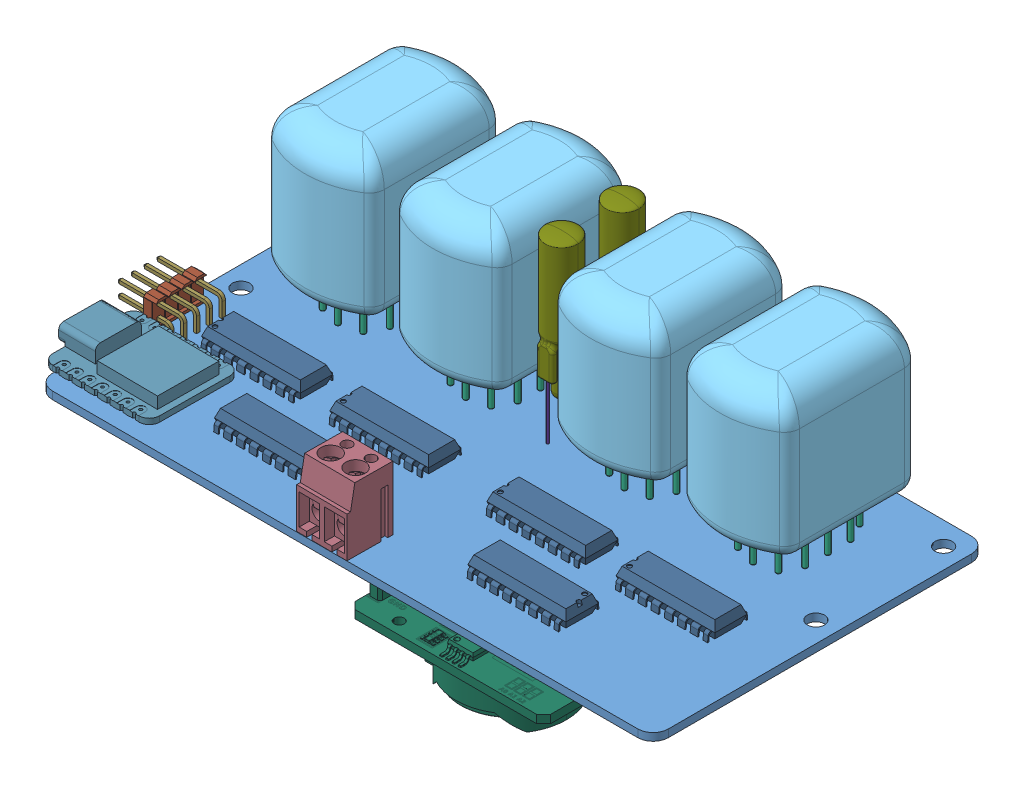
SolidWorks assembly board, configuration Défaut. Lengths in mm.
Overall size (127.16 50.53 67.27).
290 component instances, 53 part files, 23 mates.
Components (placement in the parent):
- pcb-1: pcb [Défaut] at origin size (121.6 1.5 65.9)
- IN-12A.stp-1: IN-12A.stp [Défaut] at (-40.9487 32.5 -15.5981) x (0 1 0) z (1 0 0) size (35 31 21)
  - 2.stp-1: 2.stp [Défaut] at origin size (2.7 24.17 15.83)
  - 3.stp-1: 3.stp [Défaut] at (-12.2 0 0) x (0 0 -1) z (-1 0 0) size (2 1.5 18.5)
  - 4.stp-1: 4.stp [Défaut] at (-12.2 0 0) x (0 0 1) z (-1 0 0) size (2 1.5 18.5)
  - 5.stp-1: 5.stp [Défaut] at (-12 0 0) x (0 0 -1) z (1 0 0) size (2.1 2.1 1)
  - 5.stp-2: 5.stp [Défaut] at (-10.8 0 0) x (0 0 -1) z (1 0 0) size (2.1 2.1 1)
  - 5.stp-3: 5.stp [Défaut] at (-9.6 0 0) x (0 0 -1) z (1 0 0) size (2.1 2.1 1)
  - 5.stp-4: 5.stp [Défaut] at (-8.4 0 0) x (0 0 -1) z (1 0 0) size (2.1 2.1 1)
  - 5.stp-5: 5.stp [Défaut] at (-7.2 0 0) x (0 0 -1) z (1 0 0) size (2.1 2.1 1)
  - 5.stp-6: 5.stp [Défaut] at (-6 0 0) x (0 0 -1) z (1 0 0) size (2.1 2.1 1)
  - 5.stp-7: 5.stp [Défaut] at (-4.8 0 0) x (0 0 -1) z (1 0 0) size (2.1 2.1 1)
  - 5.stp-8: 5.stp [Défaut] at (-3.6 0 0) x (0 0 -1) z (1 0 0) size (2.1 2.1 1)
  - 5.stp-9: 5.stp [Défaut] at (-2.4 0 0) x (0 0 -1) z (1 0 0) size (2.1 2.1 1)
  - 5.stp-10: 5.stp [Défaut] at (-1.2 0 0) x (0 0 -1) z (1 0 0) size (2.1 2.1 1)
  - 6.stp-1: 6.stp [Défaut] at (-11 16.1596 7.8778) x (0 -0.787778 0.61596) z (-1 0 0) size (2.1 2.1 1)
  - 7.stp-1: 7.stp [Défaut] at (-9.8 16.1596 7.8778) x (0 -0.787778 0.61596) z (-1 0 0) size (2.1 2.1 1)
  - 8.stp-1: 8.stp [Défaut] at (-8.6 16.1596 7.8778) x (0 -0.787778 0.61596) z (-1 0 0) size (2.1 2.1 1)
  - 9.stp-1: 9.stp [Défaut] at (-7.4 16.1596 7.8778) x (0 -0.787778 0.61596) z (-1 0 0) size (2.1 2.1 1)
  - 10.stp-1: 10.stp [Défaut] at (-6.2 16.1596 7.8778) x (0 -0.787778 0.61596) z (-1 0 0) size (2.1 2.1 1)
  - 11.stp-1: 11.stp [Défaut] at (-5 16.1596 7.8778) x (0 -0.787778 0.61596) z (-1 0 0) size (2.1 2.1 1)
  - 12.stp-1: 12.stp [Défaut] at (-3.8 16.1596 7.8778) x (0 -0.787778 0.61596) z (-1 0 0) size (2.1 2.1 1)
  - 13.stp-1: 13.stp [Défaut] at (-2.6 16.1596 7.8778) x (0 -0.787778 0.61596) z (-1 0 0) size (2.1 2.1 1)
  - 14.stp-1: 14.stp [Défaut] at (-1.4 16.1596 7.8778) x (0 -0.787778 0.61596) z (-1 0 0) size (2.1 2.1 1)
  - 15.stp-1: 15.stp [Défaut] at (-0.2 16.1596 7.8778) x (0 -0.787778 0.61596) z (-1 0 0) size (2.1 2.1 1)
  - 5.stp-11: 5.stp [Défaut] x (0 0 -1) z (1 0 0) size (2.1 2.1 1)
  - 5.stp-12: 5.stp [Défaut] at (-13.2 0 0) x (0 0 -1) z (1 0 0) size (2.1 2.1 1)
  - 16.stp-1: 16.stp [Défaut] at (1 16.1596 7.8778) x (0 -0.787778 0.61596) z (-1 0 0) size (2.1 2.1 1)
  - 17.stp-1: 17.stp [Défaut] at (-12.2 16.1596 7.8778) x (0 -0.787778 0.61596) z (-1 0 0) size (2.1 2.1 1)
  - 18.stp-1: 18.stp [Défaut] at (-13.2 0 0) x (0 0 -1) z (-1 0 0) size (15.83 24.17 12.28)
  - 19.stp-1: 19.stp [Défaut] x (1 0 0) z (0 1 0) size (1.51 1.46 20.68)
  - 20.stp-1: 20.stp [Défaut] at (1 0 0) size (4 22.27 2.42)
  - 21.stp-1: 21.stp [Défaut] at (-13.4 0 0) x (0 0 -1) z (-1 0 0) size (15.83 24.17 1)
  - 22.stp-1: 22.stp [Défaut] at (-14.4 0 0) x (0 0 -1) z (-1 0 0) size (15.83 27.29 2)
  - 23.stp-1: 23.stp [Défaut] x (0 0 -1) z (-1 0 0) size (21 31 33)
  - 24.stp-1: 24.stp [Défaut] x (0 0 -1) z (-1 0 0) size (1 1 15.5)
  - 24.stp-2: 24.stp [Défaut] at (0 -4.5 0) x (0 0 -1) z (-1 0 0) size (1 1 15.5)
  - 24.stp-3: 24.stp [Défaut] at (0 -8 -1.75) x (0 0 -1) z (-1 0 0) size (1 1 15.5)
  - 24.stp-4: 24.stp [Défaut] at (0 -9 -5.75) x (0 0 -1) z (-1 0 0) size (1 1 15.5)
  - 24.stp-5: 24.stp [Défaut] at (0 -8 -9.75) x (0 0 -1) z (-1 0 0) size (1 1 15.5)
  - 24.stp-6: 24.stp [Défaut] at (0 -4.5 -11.5) x (0 0 -1) z (-1 0 0) size (1 1 15.5)
  - 24.stp-7: 24.stp [Défaut] at (0 0 -11.5) x (0 0 -1) z (-1 0 0) size (1 1 15.5)
  - 24.stp-8: 24.stp [Défaut] at (0 4.5 -11.5) x (0 0 -1) z (-1 0 0) size (1 1 15.5)
  - 24.stp-9: 24.stp [Défaut] at (0 8 -9.75) x (0 0 -1) z (-1 0 0) size (1 1 15.5)
  - 24.stp-10: 24.stp [Défaut] at (0 9 -5.75) x (0 0 -1) z (-1 0 0) size (1 1 15.5)
  - 24.stp-11: 24.stp [Défaut] at (0 8 -1.75) x (0 0 -1) z (-1 0 0) size (1 1 15.5)
  - 24.stp-12: 24.stp [Défaut] at (0 4.5 0) x (0 0 -1) z (-1 0 0) size (1 1 15.5)
  - 25.stp-1: 25.stp [Défaut] at (-1.4 0 0) x (0 0 1) z (1 0 0) size (10.55 22 0.2)
  - 26.stp-1: 26.stp [Défaut] at (-2.6 0 0) x (0 0 1) z (1 0 0) size (11 22 0.2)
  - 27.stp-1: 27.stp [Défaut] at (-3.8 0 0) x (0 0 1) z (1 0 0) size (11 22 0.2)
  - 28.stp-1: 28.stp [Défaut] at (-5 0 0) x (0 0 1) z (1 0 0) size (10 22 0.2)
  - 29.stp-1: 29.stp [Défaut] at (-7.4 0 0) x (0 0 1) z (1 0 0) size (10 22 0.2)
  - 30.stp-1: 30.stp [Défaut] at (-9.6 0 0) x (0 0 -1) z (-1 0 0) size (10 22 0.2)
  - 31.stp-1: 31.stp [Défaut] at (-11 0 0) x (0 0 1) z (1 0 0) size (11 22 0.2)
  - 32.stp-1: 32.stp [Défaut] at (-12.2 0 0) x (0 0 1) z (1 0 0) size (2 22 0.2)
  - 33.stp-1: 33.stp [Défaut] at (-6 0 0) x (0 0 -1) z (-1 0 0) size (11 22 0.2)
  - 34.stp-1: 34.stp [Défaut] at (-8.6 0 0) x (0 0 1) z (1 0 0) size (10 22 0.2)
  - 1.stp-1: 1.stp [Défaut] at origin size (7.54 3.19 3.19)
  - 1-0.stp-1: 1-0.stp [Défaut] at origin size (11.99 9.11 6.32)
  - 1-1.stp-1: 1-1.stp [Défaut] at origin size (5.03 4.26 4.61)
  - 1-2.stp-1: 1-2.stp [Défaut] at origin size (8.17 8.42 6.65)
  - 1-3.stp-1: 1-3.stp [Défaut] at origin size (17.22 12.89 7.69)
  - 1-4.stp-1: 1-4.stp [Défaut] at origin size (13.11 12.81 7.39)
  - 1-5.stp-1: 1-5.stp [Défaut] at origin size (15.91 7.54 6.9)
  - 1-6.stp-1: 1-6.stp [Défaut] at origin size (10.39 4.47 4.23)
  - 1-7.stp-1: 1-7.stp [Défaut] at origin size (7.32 4.98 2.44)
  - 1-8.stp-1: 1-8.stp [Défaut] at origin size (10.29 4.36 5.63)
  - 1-9.stp-1: 1-9.stp [Défaut] at origin size (12.89 8.1 7.83)
- IN-12A.stp-2: IN-12A.stp [Défaut] at (15.5408 32.5 -15.6508) x (0 1 0) z (1 0 0) size (35 31 21)
  - 2.stp-1: 2.stp [Défaut] at origin size (2.7 24.17 15.83)
  - 3.stp-1: 3.stp [Défaut] at (-12.2 0 0) x (0 0 -1) z (-1 0 0) size (2 1.5 18.5)
  - 4.stp-1: 4.stp [Défaut] at (-12.2 0 0) x (0 0 1) z (-1 0 0) size (2 1.5 18.5)
  - 5.stp-1: 5.stp [Défaut] at (-12 0 0) x (0 0 -1) z (1 0 0) size (2.1 2.1 1)
  - 5.stp-2: 5.stp [Défaut] at (-10.8 0 0) x (0 0 -1) z (1 0 0) size (2.1 2.1 1)
  - 5.stp-3: 5.stp [Défaut] at (-9.6 0 0) x (0 0 -1) z (1 0 0) size (2.1 2.1 1)
  - 5.stp-4: 5.stp [Défaut] at (-8.4 0 0) x (0 0 -1) z (1 0 0) size (2.1 2.1 1)
  - 5.stp-5: 5.stp [Défaut] at (-7.2 0 0) x (0 0 -1) z (1 0 0) size (2.1 2.1 1)
  - 5.stp-6: 5.stp [Défaut] at (-6 0 0) x (0 0 -1) z (1 0 0) size (2.1 2.1 1)
  - 5.stp-7: 5.stp [Défaut] at (-4.8 0 0) x (0 0 -1) z (1 0 0) size (2.1 2.1 1)
  - 5.stp-8: 5.stp [Défaut] at (-3.6 0 0) x (0 0 -1) z (1 0 0) size (2.1 2.1 1)
  - 5.stp-9: 5.stp [Défaut] at (-2.4 0 0) x (0 0 -1) z (1 0 0) size (2.1 2.1 1)
  - 5.stp-10: 5.stp [Défaut] at (-1.2 0 0) x (0 0 -1) z (1 0 0) size (2.1 2.1 1)
  - 6.stp-1: 6.stp [Défaut] at (-11 16.1596 7.8778) x (0 -0.787778 0.61596) z (-1 0 0) size (2.1 2.1 1)
  - 7.stp-1: 7.stp [Défaut] at (-9.8 16.1596 7.8778) x (0 -0.787778 0.61596) z (-1 0 0) size (2.1 2.1 1)
  - 8.stp-1: 8.stp [Défaut] at (-8.6 16.1596 7.8778) x (0 -0.787778 0.61596) z (-1 0 0) size (2.1 2.1 1)
  - 9.stp-1: 9.stp [Défaut] at (-7.4 16.1596 7.8778) x (0 -0.787778 0.61596) z (-1 0 0) size (2.1 2.1 1)
  - 10.stp-1: 10.stp [Défaut] at (-6.2 16.1596 7.8778) x (0 -0.787778 0.61596) z (-1 0 0) size (2.1 2.1 1)
  - 11.stp-1: 11.stp [Défaut] at (-5 16.1596 7.8778) x (0 -0.787778 0.61596) z (-1 0 0) size (2.1 2.1 1)
  - 12.stp-1: 12.stp [Défaut] at (-3.8 16.1596 7.8778) x (0 -0.787778 0.61596) z (-1 0 0) size (2.1 2.1 1)
  - 13.stp-1: 13.stp [Défaut] at (-2.6 16.1596 7.8778) x (0 -0.787778 0.61596) z (-1 0 0) size (2.1 2.1 1)
  - 14.stp-1: 14.stp [Défaut] at (-1.4 16.1596 7.8778) x (0 -0.787778 0.61596) z (-1 0 0) size (2.1 2.1 1)
  - 15.stp-1: 15.stp [Défaut] at (-0.2 16.1596 7.8778) x (0 -0.787778 0.61596) z (-1 0 0) size (2.1 2.1 1)
  - 5.stp-11: 5.stp [Défaut] x (0 0 -1) z (1 0 0) size (2.1 2.1 1)
  - 5.stp-12: 5.stp [Défaut] at (-13.2 0 0) x (0 0 -1) z (1 0 0) size (2.1 2.1 1)
  - 16.stp-1: 16.stp [Défaut] at (1 16.1596 7.8778) x (0 -0.787778 0.61596) z (-1 0 0) size (2.1 2.1 1)
  - 17.stp-1: 17.stp [Défaut] at (-12.2 16.1596 7.8778) x (0 -0.787778 0.61596) z (-1 0 0) size (2.1 2.1 1)
  - 18.stp-1: 18.stp [Défaut] at (-13.2 0 0) x (0 0 -1) z (-1 0 0) size (15.83 24.17 12.28)
  - 19.stp-1: 19.stp [Défaut] x (1 0 0) z (0 1 0) size (1.51 1.46 20.68)
  - 20.stp-1: 20.stp [Défaut] at (1 0 0) size (4 22.27 2.42)
  - 21.stp-1: 21.stp [Défaut] at (-13.4 0 0) x (0 0 -1) z (-1 0 0) size (15.83 24.17 1)
  - 22.stp-1: 22.stp [Défaut] at (-14.4 0 0) x (0 0 -1) z (-1 0 0) size (15.83 27.29 2)
  - 23.stp-1: 23.stp [Défaut] x (0 0 -1) z (-1 0 0) size (21 31 33)
  - 24.stp-1: 24.stp [Défaut] x (0 0 -1) z (-1 0 0) size (1 1 15.5)
  - 24.stp-2: 24.stp [Défaut] at (0 -4.5 0) x (0 0 -1) z (-1 0 0) size (1 1 15.5)
  - 24.stp-3: 24.stp [Défaut] at (0 -8 -1.75) x (0 0 -1) z (-1 0 0) size (1 1 15.5)
  - 24.stp-4: 24.stp [Défaut] at (0 -9 -5.75) x (0 0 -1) z (-1 0 0) size (1 1 15.5)
  - 24.stp-5: 24.stp [Défaut] at (0 -8 -9.75) x (0 0 -1) z (-1 0 0) size (1 1 15.5)
  - 24.stp-6: 24.stp [Défaut] at (0 -4.5 -11.5) x (0 0 -1) z (-1 0 0) size (1 1 15.5)
  - 24.stp-7: 24.stp [Défaut] at (0 0 -11.5) x (0 0 -1) z (-1 0 0) size (1 1 15.5)
  - 24.stp-8: 24.stp [Défaut] at (0 4.5 -11.5) x (0 0 -1) z (-1 0 0) size (1 1 15.5)
  - 24.stp-9: 24.stp [Défaut] at (0 8 -9.75) x (0 0 -1) z (-1 0 0) size (1 1 15.5)
  - 24.stp-10: 24.stp [Défaut] at (0 9 -5.75) x (0 0 -1) z (-1 0 0) size (1 1 15.5)
  - 24.stp-11: 24.stp [Défaut] at (0 8 -1.75) x (0 0 -1) z (-1 0 0) size (1 1 15.5)
  - 24.stp-12: 24.stp [Défaut] at (0 4.5 0) x (0 0 -1) z (-1 0 0) size (1 1 15.5)
  - 25.stp-1: 25.stp [Défaut] at (-1.4 0 0) x (0 0 1) z (1 0 0) size (10.55 22 0.2)
  - 26.stp-1: 26.stp [Défaut] at (-2.6 0 0) x (0 0 1) z (1 0 0) size (11 22 0.2)
  - 27.stp-1: 27.stp [Défaut] at (-3.8 0 0) x (0 0 1) z (1 0 0) size (11 22 0.2)
  - 28.stp-1: 28.stp [Défaut] at (-5 0 0) x (0 0 1) z (1 0 0) size (10 22 0.2)
  - 29.stp-1: 29.stp [Défaut] at (-7.4 0 0) x (0 0 1) z (1 0 0) size (10 22 0.2)
  - 30.stp-1: 30.stp [Défaut] at (-9.6 0 0) x (0 0 -1) z (-1 0 0) size (10 22 0.2)
  - 31.stp-1: 31.stp [Défaut] at (-11 0 0) x (0 0 1) z (1 0 0) size (11 22 0.2)
  - 32.stp-1: 32.stp [Défaut] at (-12.2 0 0) x (0 0 1) z (1 0 0) size (2 22 0.2)
  - 33.stp-1: 33.stp [Défaut] at (-6 0 0) x (0 0 -1) z (-1 0 0) size (11 22 0.2)
  - 34.stp-1: 34.stp [Défaut] at (-8.6 0 0) x (0 0 1) z (1 0 0) size (10 22 0.2)
  - 1.stp-1: 1.stp [Défaut] at origin size (7.54 3.19 3.19)
  - 1-0.stp-1: 1-0.stp [Défaut] at origin size (11.99 9.11 6.32)
  - 1-1.stp-1: 1-1.stp [Défaut] at origin size (5.03 4.26 4.61)
  - 1-2.stp-1: 1-2.stp [Défaut] at origin size (8.17 8.42 6.65)
  - 1-3.stp-1: 1-3.stp [Défaut] at origin size (17.22 12.89 7.69)
  - 1-4.stp-1: 1-4.stp [Défaut] at origin size (13.11 12.81 7.39)
  - 1-5.stp-1: 1-5.stp [Défaut] at origin size (15.91 7.54 6.9)
  - 1-6.stp-1: 1-6.stp [Défaut] at origin size (10.39 4.47 4.23)
  - 1-7.stp-1: 1-7.stp [Défaut] at origin size (7.32 4.98 2.44)
  - 1-8.stp-1: 1-8.stp [Défaut] at origin size (10.29 4.36 5.63)
  - 1-9.stp-1: 1-9.stp [Défaut] at origin size (12.89 8.1 7.83)
- IN-12A.stp-3: IN-12A.stp [Défaut] at (-15.577 32.5 -15.4564) x (0 1 0) z (1 0 0) size (35 31 21)
  - 2.stp-1: 2.stp [Défaut] at origin size (2.7 24.17 15.83)
  - 3.stp-1: 3.stp [Défaut] at (-12.2 0 0) x (0 0 -1) z (-1 0 0) size (2 1.5 18.5)
  - 4.stp-1: 4.stp [Défaut] at (-12.2 0 0) x (0 0 1) z (-1 0 0) size (2 1.5 18.5)
  - 5.stp-1: 5.stp [Défaut] at (-12 0 0) x (0 0 -1) z (1 0 0) size (2.1 2.1 1)
  - 5.stp-2: 5.stp [Défaut] at (-10.8 0 0) x (0 0 -1) z (1 0 0) size (2.1 2.1 1)
  - 5.stp-3: 5.stp [Défaut] at (-9.6 0 0) x (0 0 -1) z (1 0 0) size (2.1 2.1 1)
  - 5.stp-4: 5.stp [Défaut] at (-8.4 0 0) x (0 0 -1) z (1 0 0) size (2.1 2.1 1)
  - 5.stp-5: 5.stp [Défaut] at (-7.2 0 0) x (0 0 -1) z (1 0 0) size (2.1 2.1 1)
  - 5.stp-6: 5.stp [Défaut] at (-6 0 0) x (0 0 -1) z (1 0 0) size (2.1 2.1 1)
  - 5.stp-7: 5.stp [Défaut] at (-4.8 0 0) x (0 0 -1) z (1 0 0) size (2.1 2.1 1)
  - 5.stp-8: 5.stp [Défaut] at (-3.6 0 0) x (0 0 -1) z (1 0 0) size (2.1 2.1 1)
  - 5.stp-9: 5.stp [Défaut] at (-2.4 0 0) x (0 0 -1) z (1 0 0) size (2.1 2.1 1)
  - 5.stp-10: 5.stp [Défaut] at (-1.2 0 0) x (0 0 -1) z (1 0 0) size (2.1 2.1 1)
  - 6.stp-1: 6.stp [Défaut] at (-11 16.1596 7.8778) x (0 -0.787778 0.61596) z (-1 0 0) size (2.1 2.1 1)
  - 7.stp-1: 7.stp [Défaut] at (-9.8 16.1596 7.8778) x (0 -0.787778 0.61596) z (-1 0 0) size (2.1 2.1 1)
  - 8.stp-1: 8.stp [Défaut] at (-8.6 16.1596 7.8778) x (0 -0.787778 0.61596) z (-1 0 0) size (2.1 2.1 1)
  - 9.stp-1: 9.stp [Défaut] at (-7.4 16.1596 7.8778) x (0 -0.787778 0.61596) z (-1 0 0) size (2.1 2.1 1)
  - 10.stp-1: 10.stp [Défaut] at (-6.2 16.1596 7.8778) x (0 -0.787778 0.61596) z (-1 0 0) size (2.1 2.1 1)
  - 11.stp-1: 11.stp [Défaut] at (-5 16.1596 7.8778) x (0 -0.787778 0.61596) z (-1 0 0) size (2.1 2.1 1)
  - 12.stp-1: 12.stp [Défaut] at (-3.8 16.1596 7.8778) x (0 -0.787778 0.61596) z (-1 0 0) size (2.1 2.1 1)
  - 13.stp-1: 13.stp [Défaut] at (-2.6 16.1596 7.8778) x (0 -0.787778 0.61596) z (-1 0 0) size (2.1 2.1 1)
  - 14.stp-1: 14.stp [Défaut] at (-1.4 16.1596 7.8778) x (0 -0.787778 0.61596) z (-1 0 0) size (2.1 2.1 1)
  - 15.stp-1: 15.stp [Défaut] at (-0.2 16.1596 7.8778) x (0 -0.787778 0.61596) z (-1 0 0) size (2.1 2.1 1)
  - 5.stp-11: 5.stp [Défaut] x (0 0 -1) z (1 0 0) size (2.1 2.1 1)
  - 5.stp-12: 5.stp [Défaut] at (-13.2 0 0) x (0 0 -1) z (1 0 0) size (2.1 2.1 1)
  - 16.stp-1: 16.stp [Défaut] at (1 16.1596 7.8778) x (0 -0.787778 0.61596) z (-1 0 0) size (2.1 2.1 1)
  - 17.stp-1: 17.stp [Défaut] at (-12.2 16.1596 7.8778) x (0 -0.787778 0.61596) z (-1 0 0) size (2.1 2.1 1)
  - 18.stp-1: 18.stp [Défaut] at (-13.2 0 0) x (0 0 -1) z (-1 0 0) size (15.83 24.17 12.28)
  - 19.stp-1: 19.stp [Défaut] x (1 0 0) z (0 1 0) size (1.51 1.46 20.68)
  - 20.stp-1: 20.stp [Défaut] at (1 0 0) size (4 22.27 2.42)
  - 21.stp-1: 21.stp [Défaut] at (-13.4 0 0) x (0 0 -1) z (-1 0 0) size (15.83 24.17 1)
  - 22.stp-1: 22.stp [Défaut] at (-14.4 0 0) x (0 0 -1) z (-1 0 0) size (15.83 27.29 2)
  - 23.stp-1: 23.stp [Défaut] x (0 0 -1) z (-1 0 0) size (21 31 33)
  - 24.stp-1: 24.stp [Défaut] x (0 0 -1) z (-1 0 0) size (1 1 15.5)
  - 24.stp-2: 24.stp [Défaut] at (0 -4.5 0) x (0 0 -1) z (-1 0 0) size (1 1 15.5)
  - 24.stp-3: 24.stp [Défaut] at (0 -8 -1.75) x (0 0 -1) z (-1 0 0) size (1 1 15.5)
  - 24.stp-4: 24.stp [Défaut] at (0 -9 -5.75) x (0 0 -1) z (-1 0 0) size (1 1 15.5)
  - 24.stp-5: 24.stp [Défaut] at (0 -8 -9.75) x (0 0 -1) z (-1 0 0) size (1 1 15.5)
  - 24.stp-6: 24.stp [Défaut] at (0 -4.5 -11.5) x (0 0 -1) z (-1 0 0) size (1 1 15.5)
  - 24.stp-7: 24.stp [Défaut] at (0 0 -11.5) x (0 0 -1) z (-1 0 0) size (1 1 15.5)
  - 24.stp-8: 24.stp [Défaut] at (0 4.5 -11.5) x (0 0 -1) z (-1 0 0) size (1 1 15.5)
  - 24.stp-9: 24.stp [Défaut] at (0 8 -9.75) x (0 0 -1) z (-1 0 0) size (1 1 15.5)
  - 24.stp-10: 24.stp [Défaut] at (0 9 -5.75) x (0 0 -1) z (-1 0 0) size (1 1 15.5)
  - 24.stp-11: 24.stp [Défaut] at (0 8 -1.75) x (0 0 -1) z (-1 0 0) size (1 1 15.5)
  - 24.stp-12: 24.stp [Défaut] at (0 4.5 0) x (0 0 -1) z (-1 0 0) size (1 1 15.5)
  - 25.stp-1: 25.stp [Défaut] at (-1.4 0 0) x (0 0 1) z (1 0 0) size (10.55 22 0.2)
  - 26.stp-1: 26.stp [Défaut] at (-2.6 0 0) x (0 0 1) z (1 0 0) size (11 22 0.2)
  - 27.stp-1: 27.stp [Défaut] at (-3.8 0 0) x (0 0 1) z (1 0 0) size (11 22 0.2)
  - 28.stp-1: 28.stp [Défaut] at (-5 0 0) x (0 0 1) z (1 0 0) size (10 22 0.2)
  - 29.stp-1: 29.stp [Défaut] at (-7.4 0 0) x (0 0 1) z (1 0 0) size (10 22 0.2)
  - 30.stp-1: 30.stp [Défaut] at (-9.6 0 0) x (0 0 -1) z (-1 0 0) size (10 22 0.2)
  - 31.stp-1: 31.stp [Défaut] at (-11 0 0) x (0 0 1) z (1 0 0) size (11 22 0.2)
  - 32.stp-1: 32.stp [Défaut] at (-12.2 0 0) x (0 0 1) z (1 0 0) size (2 22 0.2)
  - 33.stp-1: 33.stp [Défaut] at (-6 0 0) x (0 0 -1) z (-1 0 0) size (11 22 0.2)
  - 34.stp-1: 34.stp [Défaut] at (-8.6 0 0) x (0 0 1) z (1 0 0) size (10 22 0.2)
  - 1.stp-1: 1.stp [Défaut] at origin size (7.54 3.19 3.19)
  - 1-0.stp-1: 1-0.stp [Défaut] at origin size (11.99 9.11 6.32)
  - 1-1.stp-1: 1-1.stp [Défaut] at origin size (5.03 4.26 4.61)
  - 1-2.stp-1: 1-2.stp [Défaut] at origin size (8.17 8.42 6.65)
  - 1-3.stp-1: 1-3.stp [Défaut] at origin size (17.22 12.89 7.69)
  - 1-4.stp-1: 1-4.stp [Défaut] at origin size (13.11 12.81 7.39)
  - 1-5.stp-1: 1-5.stp [Défaut] at origin size (15.91 7.54 6.9)
  - 1-6.stp-1: 1-6.stp [Défaut] at origin size (10.39 4.47 4.23)
  - 1-7.stp-1: 1-7.stp [Défaut] at origin size (7.32 4.98 2.44)
  - 1-8.stp-1: 1-8.stp [Défaut] at origin size (10.29 4.36 5.63)
  - 1-9.stp-1: 1-9.stp [Défaut] at origin size (12.89 8.1 7.83)
- IN-12A.stp-4: IN-12A.stp [Défaut] at (40.934 32.5 -15.666) x (0 1 0) z (1 0 0) size (35 31 21)
  - 2.stp-1: 2.stp [Défaut] at origin size (2.7 24.17 15.83)
  - 3.stp-1: 3.stp [Défaut] at (-12.2 0 0) x (0 0 -1) z (-1 0 0) size (2 1.5 18.5)
  - 4.stp-1: 4.stp [Défaut] at (-12.2 0 0) x (0 0 1) z (-1 0 0) size (2 1.5 18.5)
  - 5.stp-1: 5.stp [Défaut] at (-12 0 0) x (0 0 -1) z (1 0 0) size (2.1 2.1 1)
  - 5.stp-2: 5.stp [Défaut] at (-10.8 0 0) x (0 0 -1) z (1 0 0) size (2.1 2.1 1)
  - 5.stp-3: 5.stp [Défaut] at (-9.6 0 0) x (0 0 -1) z (1 0 0) size (2.1 2.1 1)
  - 5.stp-4: 5.stp [Défaut] at (-8.4 0 0) x (0 0 -1) z (1 0 0) size (2.1 2.1 1)
  - 5.stp-5: 5.stp [Défaut] at (-7.2 0 0) x (0 0 -1) z (1 0 0) size (2.1 2.1 1)
  - 5.stp-6: 5.stp [Défaut] at (-6 0 0) x (0 0 -1) z (1 0 0) size (2.1 2.1 1)
  - 5.stp-7: 5.stp [Défaut] at (-4.8 0 0) x (0 0 -1) z (1 0 0) size (2.1 2.1 1)
  - 5.stp-8: 5.stp [Défaut] at (-3.6 0 0) x (0 0 -1) z (1 0 0) size (2.1 2.1 1)
  - 5.stp-9: 5.stp [Défaut] at (-2.4 0 0) x (0 0 -1) z (1 0 0) size (2.1 2.1 1)
  - 5.stp-10: 5.stp [Défaut] at (-1.2 0 0) x (0 0 -1) z (1 0 0) size (2.1 2.1 1)
  - 6.stp-1: 6.stp [Défaut] at (-11 16.1596 7.8778) x (0 -0.787778 0.61596) z (-1 0 0) size (2.1 2.1 1)
  - 7.stp-1: 7.stp [Défaut] at (-9.8 16.1596 7.8778) x (0 -0.787778 0.61596) z (-1 0 0) size (2.1 2.1 1)
  - 8.stp-1: 8.stp [Défaut] at (-8.6 16.1596 7.8778) x (0 -0.787778 0.61596) z (-1 0 0) size (2.1 2.1 1)
  - 9.stp-1: 9.stp [Défaut] at (-7.4 16.1596 7.8778) x (0 -0.787778 0.61596) z (-1 0 0) size (2.1 2.1 1)
  - 10.stp-1: 10.stp [Défaut] at (-6.2 16.1596 7.8778) x (0 -0.787778 0.61596) z (-1 0 0) size (2.1 2.1 1)
  - 11.stp-1: 11.stp [Défaut] at (-5 16.1596 7.8778) x (0 -0.787778 0.61596) z (-1 0 0) size (2.1 2.1 1)
  - 12.stp-1: 12.stp [Défaut] at (-3.8 16.1596 7.8778) x (0 -0.787778 0.61596) z (-1 0 0) size (2.1 2.1 1)
  - 13.stp-1: 13.stp [Défaut] at (-2.6 16.1596 7.8778) x (0 -0.787778 0.61596) z (-1 0 0) size (2.1 2.1 1)
  - 14.stp-1: 14.stp [Défaut] at (-1.4 16.1596 7.8778) x (0 -0.787778 0.61596) z (-1 0 0) size (2.1 2.1 1)
  - 15.stp-1: 15.stp [Défaut] at (-0.2 16.1596 7.8778) x (0 -0.787778 0.61596) z (-1 0 0) size (2.1 2.1 1)
  - 5.stp-11: 5.stp [Défaut] x (0 0 -1) z (1 0 0) size (2.1 2.1 1)
  - 5.stp-12: 5.stp [Défaut] at (-13.2 0 0) x (0 0 -1) z (1 0 0) size (2.1 2.1 1)
  - 16.stp-1: 16.stp [Défaut] at (1 16.1596 7.8778) x (0 -0.787778 0.61596) z (-1 0 0) size (2.1 2.1 1)
  - 17.stp-1: 17.stp [Défaut] at (-12.2 16.1596 7.8778) x (0 -0.787778 0.61596) z (-1 0 0) size (2.1 2.1 1)
  - 18.stp-1: 18.stp [Défaut] at (-13.2 0 0) x (0 0 -1) z (-1 0 0) size (15.83 24.17 12.28)
  - 19.stp-1: 19.stp [Défaut] x (1 0 0) z (0 1 0) size (1.51 1.46 20.68)
  - 20.stp-1: 20.stp [Défaut] at (1 0 0) size (4 22.27 2.42)
  - 21.stp-1: 21.stp [Défaut] at (-13.4 0 0) x (0 0 -1) z (-1 0 0) size (15.83 24.17 1)
  - 22.stp-1: 22.stp [Défaut] at (-14.4 0 0) x (0 0 -1) z (-1 0 0) size (15.83 27.29 2)
  - 23.stp-1: 23.stp [Défaut] x (0 0 -1) z (-1 0 0) size (21 31 33)
  - 24.stp-1: 24.stp [Défaut] x (0 0 -1) z (-1 0 0) size (1 1 15.5)
  - 24.stp-2: 24.stp [Défaut] at (0 -4.5 0) x (0 0 -1) z (-1 0 0) size (1 1 15.5)
  - 24.stp-3: 24.stp [Défaut] at (0 -8 -1.75) x (0 0 -1) z (-1 0 0) size (1 1 15.5)
  - 24.stp-4: 24.stp [Défaut] at (0 -9 -5.75) x (0 0 -1) z (-1 0 0) size (1 1 15.5)
  - 24.stp-5: 24.stp [Défaut] at (0 -8 -9.75) x (0 0 -1) z (-1 0 0) size (1 1 15.5)
  - 24.stp-6: 24.stp [Défaut] at (0 -4.5 -11.5) x (0 0 -1) z (-1 0 0) size (1 1 15.5)
  - 24.stp-7: 24.stp [Défaut] at (0 0 -11.5) x (0 0 -1) z (-1 0 0) size (1 1 15.5)
  - 24.stp-8: 24.stp [Défaut] at (0 4.5 -11.5) x (0 0 -1) z (-1 0 0) size (1 1 15.5)
  - 24.stp-9: 24.stp [Défaut] at (0 8 -9.75) x (0 0 -1) z (-1 0 0) size (1 1 15.5)
  - 24.stp-10: 24.stp [Défaut] at (0 9 -5.75) x (0 0 -1) z (-1 0 0) size (1 1 15.5)
  - 24.stp-11: 24.stp [Défaut] at (0 8 -1.75) x (0 0 -1) z (-1 0 0) size (1 1 15.5)
  - 24.stp-12: 24.stp [Défaut] at (0 4.5 0) x (0 0 -1) z (-1 0 0) size (1 1 15.5)
  - 25.stp-1: 25.stp [Défaut] at (-1.4 0 0) x (0 0 1) z (1 0 0) size (10.55 22 0.2)
  - 26.stp-1: 26.stp [Défaut] at (-2.6 0 0) x (0 0 1) z (1 0 0) size (11 22 0.2)
  - 27.stp-1: 27.stp [Défaut] at (-3.8 0 0) x (0 0 1) z (1 0 0) size (11 22 0.2)
  - 28.stp-1: 28.stp [Défaut] at (-5 0 0) x (0 0 1) z (1 0 0) size (10 22 0.2)
  - 29.stp-1: 29.stp [Défaut] at (-7.4 0 0) x (0 0 1) z (1 0 0) size (10 22 0.2)
  - 30.stp-1: 30.stp [Défaut] at (-9.6 0 0) x (0 0 -1) z (-1 0 0) size (10 22 0.2)
  - 31.stp-1: 31.stp [Défaut] at (-11 0 0) x (0 0 1) z (1 0 0) size (11 22 0.2)
  - 32.stp-1: 32.stp [Défaut] at (-12.2 0 0) x (0 0 1) z (1 0 0) size (2 22 0.2)
  - 33.stp-1: 33.stp [Défaut] at (-6 0 0) x (0 0 -1) z (-1 0 0) size (11 22 0.2)
  - 34.stp-1: 34.stp [Défaut] at (-8.6 0 0) x (0 0 1) z (1 0 0) size (10 22 0.2)
  - 1.stp-1: 1.stp [Défaut] at origin size (7.54 3.19 3.19)
  - 1-0.stp-1: 1-0.stp [Défaut] at origin size (11.99 9.11 6.32)
  - 1-1.stp-1: 1-1.stp [Défaut] at origin size (5.03 4.26 4.61)
  - 1-2.stp-1: 1-2.stp [Défaut] at origin size (8.17 8.42 6.65)
  - 1-3.stp-1: 1-3.stp [Défaut] at origin size (17.22 12.89 7.69)
  - 1-4.stp-1: 1-4.stp [Défaut] at origin size (13.11 12.81 7.39)
  - 1-5.stp-1: 1-5.stp [Défaut] at origin size (15.91 7.54 6.9)
  - 1-6.stp-1: 1-6.stp [Défaut] at origin size (10.39 4.47 4.23)
  - 1-7.stp-1: 1-7.stp [Défaut] at origin size (7.32 4.98 2.44)
  - 1-8.stp-1: 1-8.stp [Défaut] at origin size (10.29 4.36 5.63)
  - 1-9.stp-1: 1-9.stp [Défaut] at origin size (12.89 8.1 7.83)
- DIP18N.step-1: DIP18N.step [Défaut] at (-50.7835 3.7087 35.4382) x (0 0 1) z (-1 0 0) size (8.53 6.85 19.5)
- DIP18N.step-2: DIP18N.step [Défaut] at (31.1067 3.7087 35.4997) x (0 0 1) z (-1 0 0) size (8.53 6.85 19.5)
- DIP18N.step-3: DIP18N.step [Défaut] at (5.6608 3.7087 35.5611) x (0 0 1) z (-1 0 0) size (8.53 6.85 19.5)
- DIP18N.step-4: DIP18N.step [Défaut] at (-25.3559 3.7087 35.5399) x (0 0 1) z (-1 0 0) size (8.53 6.85 19.5)
- DS1022-2x4RF11.stp-1: DS1022-2x4RF11.stp [Défaut] at (-56.1796 1.5 3.5604) x (0 0 1) z (0 1 0) size (10.16 13.04 8)
  - eBom-prt0.stp-1: eBom-prt0.stp [Défaut] at origin size (10.16 2.5 5)
  - eBom-prt1.stp-1: eBom-prt1.stp [Défaut] at origin size (0.64 13.04 7.09)
  - eBom-prt1.stp-2: eBom-prt1.stp [Défaut] at (2.54 0 0) size (0.64 13.04 7.09)
  - eBom-prt1.stp-3: eBom-prt1.stp [Défaut] at (5.08 0 0) size (0.64 13.04 7.09)
  - eBom-prt1.stp-4: eBom-prt1.stp [Défaut] at (7.62 0 0) size (0.64 13.04 7.09)
- DIP18N.step-5: DIP18N.step [Défaut] at (-15.751 3.7087 -7.8923) x (0.008727 0 -0.999962) z (0.999962 0 0.008727) size (8.53 6.85 19.5)
- DIP18N.step-6: DIP18N.step [Défaut] at (34.3108 3.7087 -7.8662) x (0.008727 0 -0.999962) z (0.999962 0 0.008727) size (8.53 6.85 19.5)
- Screw Terminal Block 5mm-2: Screw Terminal Block 5mm [Valor predeterminado] at (0.4217 1.5 23.933) x (-0.999962 0 -0.008727) z (0.008727 0 -0.999962) size (10.6 16.9 9)
- Seeeduino Xiao.step-1: Seeeduino Xiao.step [Défaut] at (-88.5187 11.44 25.9289) x (-0.008727 0 0.999962) z (-0.999962 0 -0.008727) size (17.8 4.27 22.5)
- DS3231 RTC.step-1: DS3231 RTC.step [Défaut] at (21.2627 -4.62 22.922) x (1 0 0) z (0 1 0) size (44.75 22.8 13.53)
- INS1.STEP-1: INS1.STEP [Défaut] at (0 18.5 -21.8057) x (0 0 1) z (-1 0 0) size (7.01 43.17 6.51)
  - INS1-Glask_rper_01.STEP-1: INS1-Glask_rper_01.STEP [Défaut] at origin size (7.01 28.6 6.51)
  - INS1_Inlay_01.STEP-1: INS1_Inlay_01.STEP [Défaut] at (0 5.1 0) size (6 41.77 5.25)
- INS1.STEP-2: INS1.STEP [Défaut] at (0 18.5 -9.8057) x (0 0 1) z (-1 0 0) size (7.01 43.17 6.51)
  - INS1-Glask_rper_01.STEP-1: INS1-Glask_rper_01.STEP [Défaut] at origin size (7.01 28.6 6.51)
  - INS1_Inlay_01.STEP-1: INS1_Inlay_01.STEP [Défaut] at (0 5.1 0) size (6 41.77 5.25)
Mates (geometry in assembly coordinates):
- Coïncidente5: coincident anti-aligned: plane of pcb-1 through (0 1.5 0) normal (0 1 0); plane of IN-12A.stp-1/24.stp-8 through (-52.4487 1.5 -11.0981) normal (0 -1 0)
- Parallèle3: parallel aligned: plane of pcb-1 through (-60.8 1.5 -32.95) normal (-1 0 0); plane of IN-12A.stp-1/23.stp-1 through (-51.4487 36.5 -5.24) normal (-1 0 0)
- Coïncidente7: coincident anti-aligned: plane of pcb-1 through (0 1.5 0) normal (0 1 0); plane of IN-12A.stp-3/24.stp-2 through (-15.577 1.5 -19.9564) normal (0 -1 0)
- Coïncidente9: coincident anti-aligned: plane of pcb-1 through (0 1.5 0) normal (0 1 0); plane of IN-12A.stp-4/24.stp-10 through (35.184 1.5 -6.666) normal (0 -1 0)
- Parallèle5: parallel aligned: plane of IN-12A.stp-1/23.stp-1 through (-51.4487 36.5 -5.24) normal (-1 0 0); plane of IN-12A.stp-4/23.stp-1 through (30.434 36.5 -5.308) normal (-1 0 0)
- Coïncidente11: coincident anti-aligned: plane of pcb-1 through (0 1.5 0) normal (0 1 0); circle of IN-12A.stp-2/24.stp-6
- Parallèle6: parallel aligned: plane of IN-12A.stp-1/23.stp-1 through (-51.4487 36.5 -5.24) normal (-1 0 0); plane of IN-12A.stp-2/23.stp-1 through (5.0408 36.5 -5.2927) normal (-1 0 0)
- Coïncidente15: coincident anti-aligned: plane of pcb-1 through (0 1.5 0) normal (0 1 0); plane of DIP18N.step-1 through (-31.2835 1.5 4.7548) normal (0 -1 0)
- Coïncidente16: coincident anti-aligned: plane of pcb-1 through (0 1.5 0) normal (0 1 0); plane of DIP18N.step-4 through (-5.8559 1.5 4.8565) normal (0 -1 0)
- Coïncidente17: coincident anti-aligned: plane of pcb-1 through (0 1.5 0) normal (0 1 0); plane of DIP18N.step-3 through (25.1608 1.5 4.8776) normal (0 -1 0)
- Coïncidente18: coincident anti-aligned: plane of pcb-1 through (0 1.5 0) normal (0 1 0); plane of DIP18N.step-2 through (50.6067 1.5 4.8163) normal (0 -1 0)
- Coïncidente19: coincident anti-aligned: plane of pcb-1 through (0 1.5 0) normal (0 1 0); plane of DS1022-2x4RF11.stp-1/eBom-prt0.stp-1 through (-60.3596 1.5 4.2457) normal (0 -1 0)
- Parallèle7: parallel aligned: plane of pcb-1 through (-60.8 1.5 -32.95) normal (-1 0 0); plane of DS1022-2x4RF11.stp-1/eBom-prt0.stp-1 through (-60.3596 1.5 3.5604) normal (-1 0 0)
- Coïncidente21: coincident anti-aligned: plane of pcb-1 through (0 1.5 0) normal (0 1 0); plane of DIP18N.step-5 through (-35.5181 1.5 22.6198) normal (0 -1 0)
- Coïncidente22: coincident anti-aligned: plane of pcb-1 through (0 1.5 0) normal (0 1 0); plane of DIP18N.step-6 through (14.5438 1.5 22.6458) normal (0 -1 0)
- Coïncidente23: coincident anti-aligned: plane of pcb-1 through (0 1.5 0) normal (0 1 0); plane of Screw Terminal Block 5mm-2 through (-9.6565 1.5 32.8454) normal (0 -1 0)
- Distance1: distance = 2.5 mm anti-aligned: plane of Seeeduino Xiao.step-1 through (-49.894 4 23.2659) normal (0 -1 0); plane of pcb-1 through (0 1.5 0) normal (0 1 0)
- Coïncidente26: coincident aligned: plane of pcb-1 through (0 0 0) normal (1 0 0)
- Coïncidente27: coincident aligned: plane of pcb-1 through (0 0 0) normal (0 0 1)
- Coïncidente28: coincident aligned: plane of pcb-1 through (0 0 0) normal (0 1 0)
- Parallèle8: parallel anti-aligned: plane of pcb-1 through (0 0 0) normal (0 -1 0); plane of DS3231 RTC.step-1 through (21.2627 -4.62 22.922) normal (0 1 0)
- Distance2: distance = 4.62 mm anti-aligned: plane of pcb-1 through (0 0 0) normal (0 -1 0); plane of DS3231 RTC.step-1 through (21.2627 -4.62 22.922) normal (0 1 0)
- Coïncidente8: coincident aligned: plane of INS1.STEP-1 through (0 18.5 -21.8057) normal (0 1 0); plane of INS1.STEP-2 through (0 18.5 -9.8057) normal (0 1 0)
